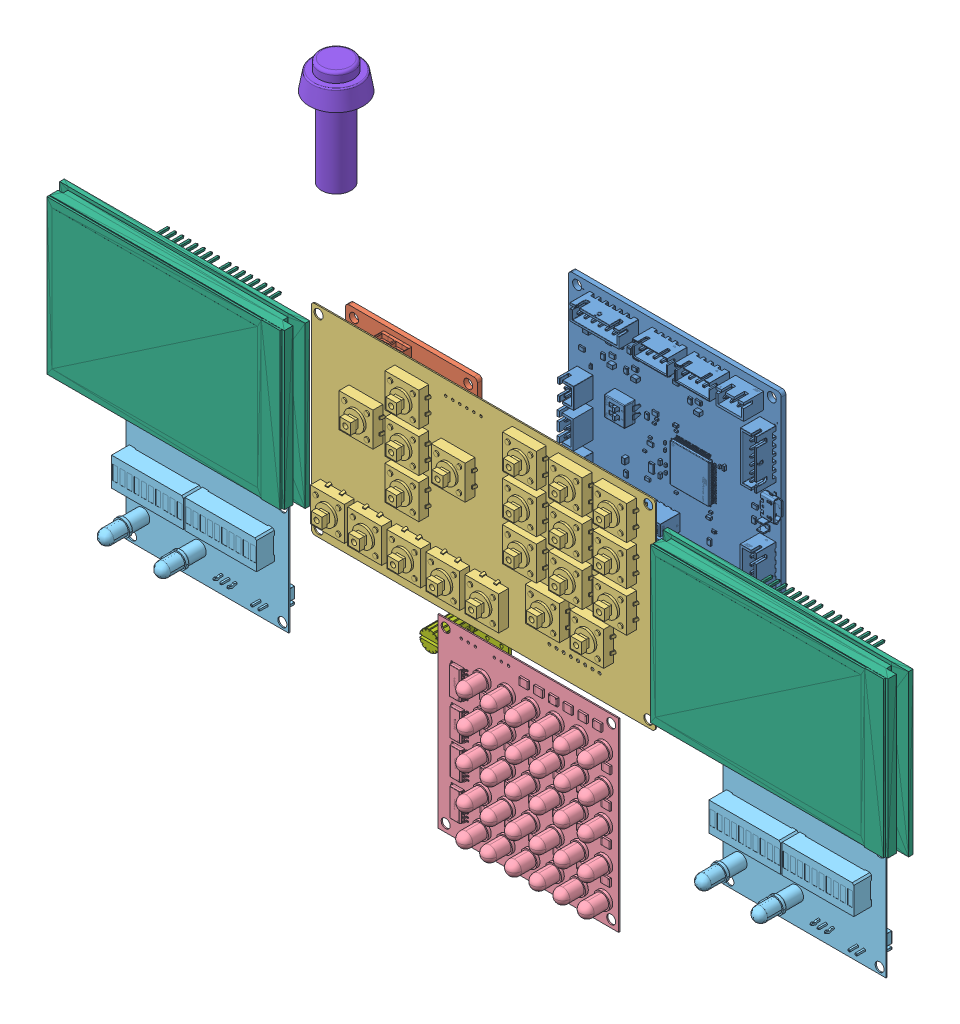
SolidWorks assembly Assembly, configuration Default. Lengths in mm.
Overall size (300.89 145.93 107.55).
11 component instances, 9 part files, 4 mates.
Components (placement in the parent):
- MCU-1: MCU [Default] at (-10.3022 6.7356 55.1454) size (75.96 70.87 10.4)
- PSU-1: PSU [Default] at (-198.7087 -101.9716 36.9881) size (46.8 37.5 15.1)
- Keypad-1: Keypad [Default] at (-66.8663 -26.3894 130.2903) size (121.92 71.12 10.8)
- LEDmatrix-1: LEDmatrix [Default] at (-92.4392 -105.2414 131.4386) size (64.13 65.66 10.01)
- LED_bars-1: LED_bars [Default] at (-43.0142 22.8012 121.1563) x (0 -1 0) z (0 0 -1) size (39.75 57.75 38.1)
- LED_bars-2: LED_bars [Default] at (168.6875 22.8012 121.1563) x (0 -1 0) z (0 0 -1) size (39.75 57.75 38.1)
- 3,5 inch display-1: 3,5 inch display [Default] at (-74.1828 63.4855 120.8159) size (87 56.9 15.4)
- 3,5 inch display-2: 3,5 inch display [Default] at (139.7063 63.4855 120.8159) size (87 56.9 15.4)
- potentiometer_B10K-1: potentiometer_B10K [Default] at (-7.1828 -8.4626 79.9687) size (17 26.43 27.6)
- power switch-1: power switch [Default] at (-88.662 95.4563 59.0798) size (19 38 19)
- DC_JACK-1: DC_JACK [Default] at (-110.0362 21.8942 73.8082) x (-1 0 0) z (0 0 -1) size (9.26 14.51 14.45)
Mates (geometry in assembly coordinates):
- Coincident2: coincident aligned: plane of 3,5 inch display-1 through (-74.1828 63.4855 136.1559) normal (0 0 1); plane of 3,5 inch display-2 through (139.7063 63.4855 136.1559) normal (0 0 1)
- Coincident3: coincident aligned: plane of 3,5 inch display-1 through (-74.1828 89.9835 120.8159) normal (0 1 0); plane of 3,5 inch display-2 through (139.7063 89.9835 120.8159) normal (0 1 0)
- Coincident4: coincident aligned: plane of LED_bars-1 through (-71.8892 2.9262 121.5677) normal (0 0 1); plane of LED_bars-2 through (139.8125 2.9262 121.5677) normal (0 0 1)
- Coincident5: coincident aligned: plane of LED_bars-1 through (-43.0142 22.8012 121.5677) normal (0 1 0); plane of LED_bars-2 through (168.6875 22.8012 121.5677) normal (0 1 0)
